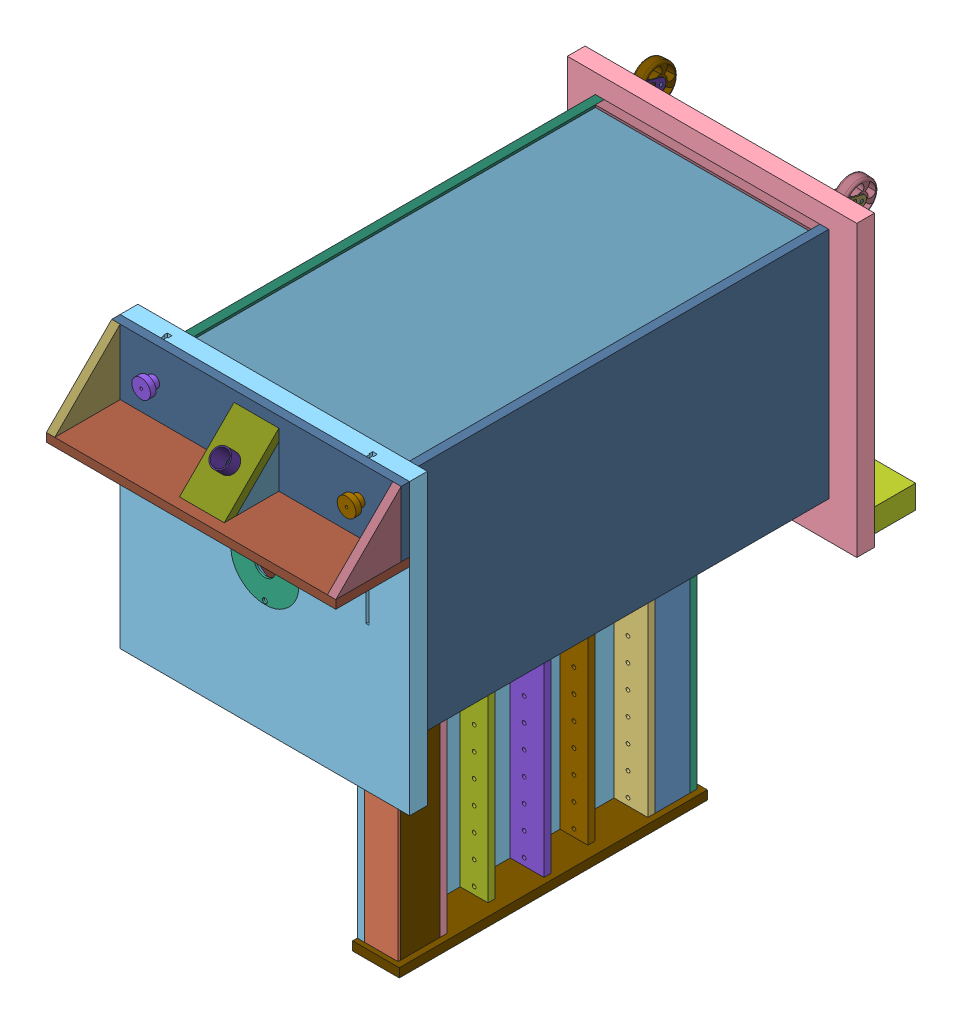
SolidWorks assembly table_petitcopeau, configuration Défaut. Lengths in mm.
Overall size (620 993.21 1253.15).
89 component instances, 72 part files, 0 mates.
Components (placement in the parent):
- table_petitcopeau.step-1: table_petitcopeau.step [Défaut] at origin size (620 993.21 1253.15)
  - E9foncer_v9.step-1: E9foncer_v9.step [Défaut] at (0 19 -19) x (1 0 0) z (0 -1 0) size (620 1140.15 624.21)
    - ROUTER ASSEMBLY v1.step-1: ROUTER ASSEMBLY v1.step [Défaut] at (0 912 0) x (1 0 0) z (0 0 -1) size (279.73 217.49 189.25)
      - ROUTER BASE.step-1: ROUTER BASE.step [Défaut] at origin size (149.23 102.91 149.22)
      - SNAP LEVER.step-1: SNAP LEVER.step [Défaut] at (-52.3627 71.9991 0) x (0.079013 0.996874 0) z (0.996874 -0.079013 0) size (32.29 26.92 12.04)
      - LOCKING TAB.step-1: LOCKING TAB.step [Défaut] at (-22.3279 76.3016 -56.7617) x (-0.917398 0 0.397971) z (0 -1 0) size (58.56 16.17 27.28)
      - SPRING TAB.step-1: SPRING TAB.step [Défaut] at (-50.6321 77.0992 0) x (-0.996601 -0.082374 0) z (0 0 -1) size (7.32 16.79 5.08)
      - Part5^ROUTER ASSEMBLY.step-1: Part5^ROUTER ASSEMBLY.step [Défaut] at (1.9997 76.3016 -52.411) x (1 0 0) z (0 -1 0) size (47.45 6 6.01)
      - ADJUST RING.step-1: ADJUST RING.step [Défaut] at (0 94.3356 0) x (0.80182 0 0.597565) z (-0.597565 0 0.80182) size (144.21 33.02 128.55)
      - MOTOR BASE.step-1: MOTOR BASE.step [Défaut] at (0 47.9951 0) x (-1 0 0) z (0 0 -1) size (111.16 203.64 116.83)
      - HANDLE.step-1: HANDLE.step [Défaut] at (65.9404 36.4291 0) x (-0.173648 0.984808 0) z (0 0 -1) size (64.76 66.04 55.9)
      - DPM 0.125x0.step-1: DPM 0.125x0.step [Défaut] at (-48.514 90.0176 16.51) x (0 0 -1) z (1 0 0) size (31.75 3.18 3.18)
      - GUIDE PLATE.step-1: GUIDE PLATE.step [Défaut] at (0 -3.175 0) x (-1 0 0) z (0 0 -1) size (149.22 3.18 149.22)
      - SNAP LEVER.step-2: SNAP LEVER.step [Défaut] at (51.516 71.8388 0) x (-0.032315 0.999478 0) z (-0.999478 -0.032315 0) size (32.29 26.92 12.04)
      - SPRING TAB.step-2: SPRING TAB.step [Défaut] at (50.6321 77.0992 0) x (0.996601 -0.082374 0) z (0 0 1) size (7.32 16.79 5.08)
      - HANDLE.step-2: HANDLE.step [Défaut] at (-65.9404 36.4291 0) x (0.173648 0.984808 0) z (0 0 1) size (64.76 66.04 55.9)
      - DPM 0.125x0.step-2: DPM 0.125x0.step [Défaut] at (48.514 90.0176 16.51) x (0 0 -1) z (1 0 0) size (31.75 3.18 3.18)
    - Assem1 v1.step-1: Assem1 v1.step [Défaut] at (150 530 -300) size (76.2 100.21 95.12)
      - Part1.step-1: Part1.step [Défaut] at (64.8109 45.9775 33.3533) size (76.2 5.08 76.2)
      - Part2.step-1: Part2.step [Défaut] at (64.8109 38.3575 33.3533) x (-0.998094 0 -0.06171) z (0.06171 0 -0.998094) size (30.99 63.5 50.8)
      - Part3.step-1: Part3.step [Défaut] at (52.1351 -2.2825 32.5696) x (0.998094 0 0.06171) z (0.059483 -0.266209 -0.962078) size (25.4 76.2 76.2)
      - Part4.step-1: Part4.step [Défaut] at (52.1351 -2.2825 32.5696) x (0.06171 0 -0.998094) z (0.998094 0 0.06171) size (15.24 15.24 30.48)
      - Part5.step-1: Part5.step [Défaut] at (65.2258 -8.5737 26.6431) size (6.35 6.35 6.35)
      - Part5.step-2: Part5.step [Défaut] at (65.3084 2.1674 25.3079) x (0.997369 0.05869 0.042559) z (0.042559 -0.949244 0.311648) size (6.35 6.35 6.35)
      - Part5.step-3: Part5.step [Défaut] at (64.7035 6.7588 35.0912) x (0.993111 0.036272 0.111421) z (0.111421 -0.586665 -0.802128) size (6.35 6.35 6.35)
      - Part5.step-4: Part5.step [Défaut] at (64.2471 -1.1445 42.4728) x (0.993111 -0.036272 0.111421) z (0.111421 0.586665 -0.802128) size (6.35 6.35 6.35)
      - Part5.step-5: Part5.step [Défaut] at (64.5699 -10.6206 37.2516) x (0.997369 -0.05869 0.042559) z (0.042559 0.949244 0.311648) size (6.35 6.35 6.35)
    - Assem1 v1(Mirror).step-1: Assem1 v1(Mirror).step [Défaut] at (-150 530 -300) x (-1 0 0) z (0 0 -1) size (76.2 100.21 95.12)
      - Part1(Mirror).step-1: Part1(Mirror).step [Défaut] at (64.8109 45.9775 -33.3533) size (76.2 5.08 76.2)
      - Part2(Mirror).step-1: Part2(Mirror).step [Défaut] at (64.8109 38.3575 -33.3533) x (-0.998094 0 0.06171) z (-0.06171 0 -0.998094) size (30.99 63.5 50.8)
      - Part3(Mirror).step-1: Part3(Mirror).step [Défaut] at (52.1351 -2.2825 -32.5696) x (0.998094 0 -0.06171) z (-0.059483 0.266209 -0.962078) size (25.4 76.2 76.2)
      - Part4(Mirror).step-1: Part4(Mirror).step [Défaut] at (52.1351 -2.2825 -32.5696) x (0.06171 0 0.998094) z (-0.998094 0 0.06171) size (15.24 15.24 30.48)
      - Part5(Mirror).step-1: Part5(Mirror).step [Défaut] at (65.2258 -8.5737 -26.6431) size (6.35 6.35 6.35)
      - Part5(Mirror).step-2: Part5(Mirror).step [Défaut] at (65.3084 2.1674 -25.3079) x (0.997369 0.05869 -0.042559) z (-0.042559 0.949244 0.311648) size (6.35 6.35 6.35)
      - Part5(Mirror).step-3: Part5(Mirror).step [Défaut] at (64.7035 6.7588 -35.0912) x (0.993111 0.036272 -0.111421) z (-0.111421 0.586665 -0.802128) size (6.35 6.35 6.35)
      - Part5(Mirror).step-4: Part5(Mirror).step [Défaut] at (64.2471 -1.1445 -42.4728) x (0.993111 -0.036272 -0.111421) z (-0.111421 -0.586665 -0.802128) size (6.35 6.35 6.35)
      - Part5(Mirror).step-5: Part5(Mirror).step [Défaut] at (64.5699 -10.6206 -37.2516) x (0.997369 -0.05869 -0.042559) z (-0.042559 -0.949244 0.311648) size (6.35 6.35 6.35)
    - 19MMBL v1.step-1: 19MMBL v1.step [Défaut] at (259.7504 850 190) x (-1 0 0) z (0 0 -1) size (35.32 22 22)
    - E9foncer_v9-0.step-1: E9foncer_v9-0.step [Défaut] at origin size (620 38 620)
    - E9foncer_v9-1.step-1: E9foncer_v9-1.step [Défaut] at origin size (620 38 620)
    - E9foncer_v9-2.step-1: E9foncer_v9-2.step [Défaut] at origin size (146.77 4 146.77)
    - E9foncer_v9-3.step-1: E9foncer_v9-3.step [Défaut] at origin size (620 88 50)
    - E9foncer_v9-4.step-1: E9foncer_v9-4.step [Défaut] at origin size (40 27 40)
    - E9foncer_v9-5.step-1: E9foncer_v9-5.step [Défaut] at origin size (40 27 40)
  - Untitled.step-1: Untitled.step [Défaut] at origin size (19 500 920)
  - Untitled-6.step-1: Untitled-6.step [Défaut] at origin size (462 120 19)
  - Untitled-7.step-1: Untitled-7.step [Défaut] at origin size (462 120 19)
  - Untitled-8.step-1: Untitled-8.step [Défaut] at origin size (462 120 19)
  - Untitled-9.step-1: Untitled-9.step [Défaut] at origin size (482 5 882)
  - Untitled-10.step-1: Untitled-10.step [Défaut] at origin size (19 500 920)
  - Untitled-11.step-1: Untitled-11.step [Défaut] at origin size (462 489 19)
  - Untitled-12.step-1: Untitled-12.step [Défaut] at origin size (462 120 19)
  - Untitled-13.step-1: Untitled-13.step [Défaut] at origin size (459 19 200)
  - Untitled-14.step-1: Untitled-14.step [Défaut] at origin size (15 455 170)
  - Untitled-15.step-1: Untitled-15.step [Défaut] at origin size (15 455 170)
  - Untitled-16.step-1: Untitled-16.step [Défaut] at origin size (436.6 15 170)
  - Untitled-17.step-1: Untitled-17.step [Défaut] at origin size (406.6 455 15)
  - Untitled-18.step-1: Untitled-18.step [Défaut] at origin size (100 19 660)
  - Untitled-19.step-1: Untitled-19.step [Défaut] at origin size (72.3 435 15)
  - Untitled-20.step-1: Untitled-20.step [Défaut] at origin size (72.3 435 15)
  - Untitled-21.step-1: Untitled-21.step [Défaut] at origin size (72.3 435 15)
  - Untitled-22.step-1: Untitled-22.step [Défaut] at origin size (15 435 85)
  - Untitled-23.step-1: Untitled-23.step [Défaut] at origin size (15 435 85)
  - Untitled-24.step-1: Untitled-24.step [Défaut] at origin size (15 435 640)
  - Untitled-25.step-1: Untitled-25.step [Défaut] at origin size (87.3 15 640)
  - Untitled-26.step-1: Untitled-26.step [Défaut] at origin size (59.6 434.93 15)
  - Untitled-27.step-1: Untitled-27.step [Défaut] at origin size (59.6 435 15)
  - Untitled-28.step-1: Untitled-28.step [Défaut] at origin size (72.3 435 15)
  - Untitled-29.step-1: Untitled-29.step [Défaut] at origin size (72.3 435 15)
  - Untitled-30.step-1: Untitled-30.step [Défaut] at origin size (87.3 15 640)
  - Untitled-31.step-1: Untitled-31.step [Défaut] at origin size (15 435 85)
  - Untitled-32.step-1: Untitled-32.step [Défaut] at origin size (15 435 75)
  - Untitled-33.step-1: Untitled-33.step [Défaut] at origin size (72.3 435 15)
  - Untitled-34.step-1: Untitled-34.step [Défaut] at origin size (72.3 435 15)
  - Untitled-35.step-1: Untitled-35.step [Défaut] at origin size (72.3 435 15)
  - Untitled-36.step-1: Untitled-36.step [Défaut] at origin size (15 435 640)
  - Untitled-37.step-1: Untitled-37.step [Défaut] at origin size (72.3 435 15)
  - Untitled-38.step-1: Untitled-38.step [Défaut] at origin size (59.6 435 15)
  - Untitled-39.step-1: Untitled-39.step [Défaut] at origin size (72.3 435 15)
  - Untitled-40.step-1: Untitled-40.step [Défaut] at origin size (59.6 434.93 15)
  - Untitled-41.step-1: Untitled-41.step [Défaut] at origin size (620 140 18)
  - Untitled-42.step-1: Untitled-42.step [Défaut] at origin size (620 18 158)
  - Untitled-43.step-1: Untitled-43.step [Défaut] at origin size (18 140 140)
  - Untitled-44.step-1: Untitled-44.step [Défaut] at origin size (18 140 140)
  - Untitled-45.step-1: Untitled-45.step [Défaut] at origin size (18 91.52 91.52)
  - Untitled-46.step-1: Untitled-46.step [Défaut] at origin size (18 91.52 91.52)
  - Untitled-47.step-1: Untitled-47.step [Défaut] at origin size (96 116.97 116.97)
  - Untitled-48.step-1: Untitled-48.step [Défaut] at origin size (40 60.1 60.1)
  - Untitled-49.step-1: Untitled-49.step [Défaut] at origin size (100 19 660)
